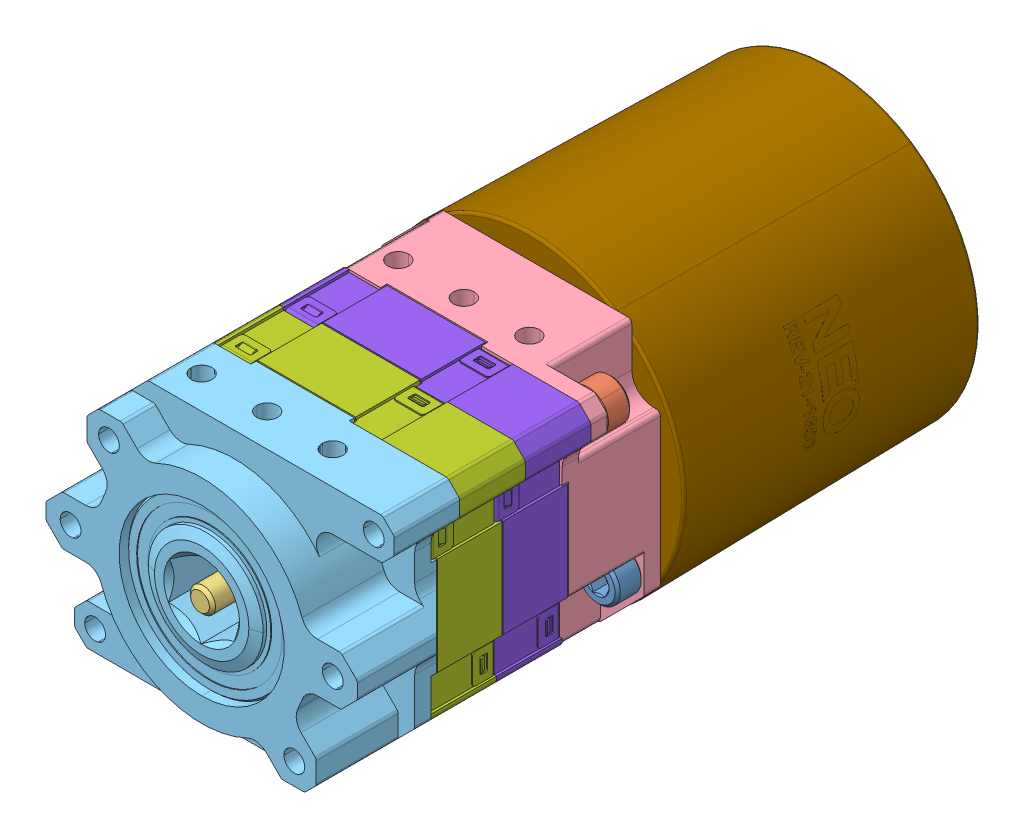
SolidWorks assembly MAXPlanetary 2-Stage, configuration Default. Lengths in mm.
Overall size (89.61 89.51 122.08).
14 component instances, 9 part files, 0 mates.
Components (placement in the parent):
- MAXPlanetary 2-Stage.STEP-1: MAXPlanetary 2-Stage.STEP [Default] at origin size (89.61 89.51 122.08)
  - REV-25-2109_2-Stage (No Shaft, For NEO).STEP-1: REV-25-2109_2-Stage (No Shaft, For NEO).STEP [Default] at origin size (65.15 54.03 73.34)
    - REV-25-2107_2-Stage.STEP-1: REV-25-2107_2-Stage.STEP [Default] at (0 0 6.35) x (-1 0 0) z (0 0 -1) size (65.15 54.03 73.34)
      - #10 Socket Head Cap Screws_0.500in Long.STEP-1: #10 Socket Head Cap Screws_0.500in Long.STEP [Default] at (21.1355 14.0872 12.7) x (0.923728 0.383049 0) z (0.383049 -0.923728 0) size (7.94 17.53 7.94)
      - #10 Socket Head Cap Screws_0.500in Long.STEP-2: #10 Socket Head Cap Screws_0.500in Long.STEP [Default] at (-21.1355 -14.0872 12.7) x (0.923728 0.383049 0) z (0.383049 -0.923728 0) size (7.94 17.53 7.94)
      - #10 Socket Head Cap Screws_1.500in Long.STEP-1: #10 Socket Head Cap Screws_1.500in Long.STEP [Default] at (-26.9919 21.4312 0) x (0.777574 0.628792 0) z (-0.628792 0.777574 0) size (7.94 42.93 7.94)
      - #10 Socket Head Cap Screws_1.500in Long.STEP-2: #10 Socket Head Cap Screws_1.500in Long.STEP [Default] at (26.9919 -21.4312 0) x (0.777574 0.628792 0) z (-0.628792 0.777574 0) size (7.94 42.93 7.94)
      - #10-32 Button Head Cap Screws_0.500in Long.STEP-1: #10-32 Button Head Cap Screws_0.500in Long.STEP [Default] at (0 0 -35.2425) x (0.655967 -0.754789 0) z (-0.754789 -0.655967 0) size (9.17 15.27 9.17)
    - REV-21-2106.STEP-1: REV-21-2106.STEP [Default] at origin size (61.91 50.8 19.05)
    - REV-21-2104.STEP-1: REV-21-2104.STEP [Default] at (0 0 44.45) x (0 0 1) z (-1 0 0) size (23.2 50.8 61.92)
    - REV-21-2108.STEP-1: REV-21-2108.STEP [Default] at (0 0 7.0985) x (-0.554615 -0.832107 0) z (0 0 -1) size (25.4 25.4 14.94)
  - REV-21-2101.STEP-1: REV-21-2101.STEP [Default] at (0 0 28.575) size (61.91 50.8 16.85)
  - REV-21-2102.STEP-1: REV-21-2102.STEP [Default] at (0 0 15.875) size (61.91 50.8 17.5)
  - REV-21-1650.STEP-1: REV-21-1650.STEP [Default] at (0 0 -9.525) x (0.554615 0.832107 0) z (0 0 1) size (64.41 64.76 93.26)
